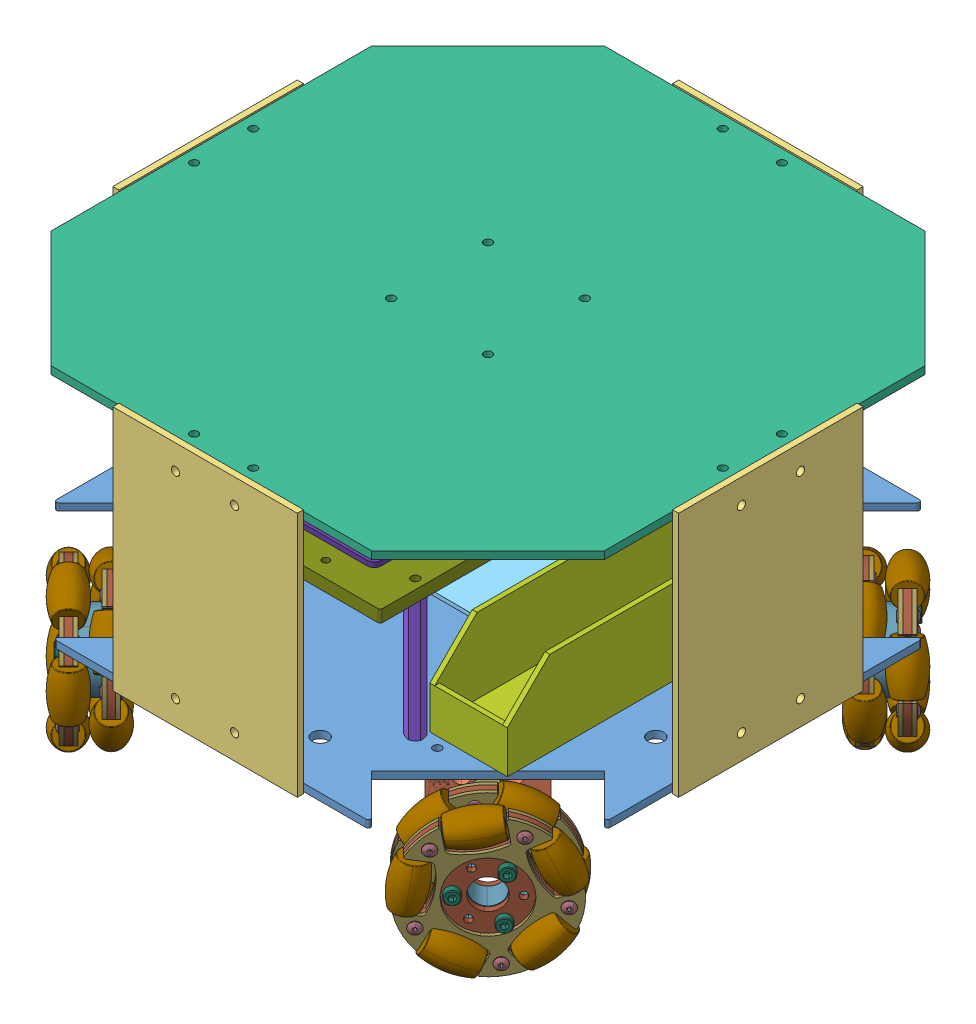
SolidWorks assembly ouijabot, configuration Default. Lengths in mm. (continued)
Components (placement in the parent): (continued)
- tx2-carrier-orbitty-1: tx2-carrier-orbitty [Default] at (43.5 74 -33.48) x (-1 0 0) z (0 -1 0) size (87.04 52.68 23.65) (continued)
  - ASG003_3D_MODEL.step-1: ASG003_3D_MODEL.step [Default] at origin size (87.04 52.68 23.65) (continued)
    - D8.step-1: D8.step [Default] at origin size (1.1 0.7 0.55) (continued)
      - 870944480.step-1: 870944480.step [Default] at (76.885 41.857 0) size (1.1 0.7 0.55) (continued)
        - Extruded-30.step-1: Extruded-30.step [Default] at origin size (1.1 0.7 0.55)
    - D7.step-1: D7.step [Default] at origin size (1 0.8 0.5)
      - 870940960.step-1: 870940960.step [Default] at (74.4974 43.1524 0) size (1 0.8 0.5)
        - Extruded-31.step-1: Extruded-31.step [Default] at origin size (1 0.8 0.5)
    - D6.step-1: D6.step [Default] at origin size (1 0.8 0.5)
      - 870940960.step-1: 870940960.step [Default] at (41.166 32.031 0) size (1 0.8 0.5)
        - Extruded-31.step-1: Extruded-31.step [Default] at origin size (1 0.8 0.5)
    - D5.step-1: D5.step [Default] at origin size (1 0.8 0.5)
      - 870940960.step-1: 870940960.step [Default] at (35.166 32.031 0) size (1 0.8 0.5)
        - Extruded-31.step-1: Extruded-31.step [Default] at origin size (1 0.8 0.5)
    - D4.step-1: D4.step [Default] at origin size (1 0.8 0.5)
      - 870940960.step-1: 870940960.step [Default] at (44.881 32.031 0) size (1 0.8 0.5)
        - Extruded-31.step-1: Extruded-31.step [Default] at origin size (1 0.8 0.5)
    - D2.step-1: D2.step [Default] at origin size (1.02 0.52 0.36)
      - 870944640.step-1: 870944640.step [Default] at (10.9212 1.0646 0) size (1.01 0.51 0.36)
        - Extruded-28.step-1: Extruded-28.step [Default] at origin size (1.01 0.51 0.36)
      - 870940480.step-1: 870940480.step [Default] at (10.4912 1.0646 0) size (0.16 0.52 0.35)
        - Extruded.step-1: Extruded.step [Default] at origin size (0.16 0.52 0.35)
      - 870940480.step-2: 870940480.step [Default] at (11.3512 1.0646 0) size (0.16 0.52 0.35)
        - Extruded.step-1: Extruded.step [Default] at origin size (0.16 0.52 0.35)
    - C57.step-1: C57.step [Default] at origin size (1.3 2.04 0.45)
      - 740904480.step-1: 740904480.step [Default] at (69.215 27.686 0) size (1.25 2 0.45)
        - Extruded-32.step-1: Extruded-32.step [Default] at origin size (1.25 2 0.45)
      - 740902240.step-1: 740902240.step [Default] at (69.215 26.7735 0) size (1.3 0.23 0.45)
        - Extruded-33.step-1: Extruded-33.step [Default] at origin size (1.3 0.23 0.45)
      - 740902240.step-2: 740902240.step [Default] at (69.215 28.586 0) size (1.3 0.23 0.45)
        - Extruded-33.step-1: Extruded-33.step [Default] at origin size (1.3 0.23 0.45)
    - C47.step-1: C47.step [Default] at origin size (1.3 2.04 0.45)
      - 740902240.step-1: 740902240.step [Default] at (72.8972 21.3736 0) size (1.3 0.23 0.45)
        - Extruded-33.step-1: Extruded-33.step [Default] at origin size (1.3 0.23 0.45)
      - 740902240.step-2: 740902240.step [Default] at (72.8972 23.1861 0) size (1.3 0.23 0.45)
        - Extruded-33.step-1: Extruded-33.step [Default] at origin size (1.3 0.23 0.45)
      - 740904480.step-1: 740904480.step [Default] at (72.8972 22.2736 0) size (1.25 2 0.45)
        - Extruded-32.step-1: Extruded-32.step [Default] at origin size (1.25 2 0.45)
    - C46.step-1: C46.step [Default] at origin size (1.3 2.04 0.45)
      - 740902240.step-1: 740902240.step [Default] at (76.9612 21.3736 0) size (1.3 0.23 0.45)
        - Extruded-33.step-1: Extruded-33.step [Default] at origin size (1.3 0.23 0.45)
      - 740902240.step-2: 740902240.step [Default] at (76.9612 23.1861 0) size (1.3 0.23 0.45)
        - Extruded-33.step-1: Extruded-33.step [Default] at origin size (1.3 0.23 0.45)
      - 740904480.step-1: 740904480.step [Default] at (76.9612 22.2736 0) size (1.25 2 0.45)
        - Extruded-32.step-1: Extruded-32.step [Default] at origin size (1.25 2 0.45)
    - C45.step-1: C45.step [Default] at origin size (1.3 2.04 0.45)
      - 740902240.step-1: 740902240.step [Default] at (74.9292 21.3736 0) size (1.3 0.23 0.45)
        - Extruded-33.step-1: Extruded-33.step [Default] at origin size (1.3 0.23 0.45)
      - 740902240.step-2: 740902240.step [Default] at (74.9292 23.1861 0) size (1.3 0.23 0.45)
        - Extruded-33.step-1: Extruded-33.step [Default] at origin size (1.3 0.23 0.45)
      - 740904480.step-1: 740904480.step [Default] at (74.9292 22.2736 0) size (1.25 2 0.45)
        - Extruded-32.step-1: Extruded-32.step [Default] at origin size (1.25 2 0.45)
    - C44.step-1: C44.step [Default] at origin size (1.02 0.52 0.36)
      - 870940480.step-1: 870940480.step [Default] at (29.084 26.6678 0) size (0.16 0.52 0.35)
        - Extruded.step-1: Extruded.step [Default] at origin size (0.16 0.52 0.35)
      - 870940480.step-2: 870940480.step [Default] at (29.944 26.6678 0) size (0.16 0.52 0.35)
        - Extruded.step-1: Extruded.step [Default] at origin size (0.16 0.52 0.35)
      - 870940640.step-1: 870940640.step [Default] at (29.514 26.6678 0) size (1.01 0.51 0.36)
        - Extruded-0.step-1: Extruded-0.step [Default] at origin size (1.01 0.51 0.36)
    - C43.step-1: C43.step [Default] at origin size (1.02 0.52 0.36)
      - 870940480.step-1: 870940480.step [Default] at (76.455 43 0) size (0.16 0.52 0.35)
        - Extruded.step-1: Extruded.step [Default] at origin size (0.16 0.52 0.35)
      - 870940480.step-2: 870940480.step [Default] at (77.315 43 0) size (0.16 0.52 0.35)
        - Extruded.step-1: Extruded.step [Default] at origin size (0.16 0.52 0.35)
      - 870940640.step-1: 870940640.step [Default] at (76.885 43 0) size (1.01 0.51 0.36)
        - Extruded-0.step-1: Extruded-0.step [Default] at origin size (1.01 0.51 0.36)
    - C42.step-1: C42.step [Default] at origin size (1.02 0.52 0.36)
      - 870940480.step-1: 870940480.step [Default] at (76.455 44.016 0) size (0.16 0.52 0.35)
        - Extruded.step-1: Extruded.step [Default] at origin size (0.16 0.52 0.35)
      - 870940480.step-2: 870940480.step [Default] at (77.315 44.016 0) size (0.16 0.52 0.35)
        - Extruded.step-1: Extruded.step [Default] at origin size (0.16 0.52 0.35)
      - 870940640.step-1: 870940640.step [Default] at (76.885 44.016 0) size (1.01 0.51 0.36)
        - Extruded-0.step-1: Extruded-0.step [Default] at origin size (1.01 0.51 0.36)
    - C41.step-1: C41.step [Default] at origin size (1.02 0.52 0.36)
      - 870940480.step-1: 870940480.step [Default] at (68.835 44.143 0) size (0.16 0.52 0.35)
        - Extruded.step-1: Extruded.step [Default] at origin size (0.16 0.52 0.35)
      - 870940480.step-2: 870940480.step [Default] at (69.695 44.143 0) size (0.16 0.52 0.35)
        - Extruded.step-1: Extruded.step [Default] at origin size (0.16 0.52 0.35)
      - 870940640.step-1: 870940640.step [Default] at (69.265 44.143 0) size (1.01 0.51 0.36)
        - Extruded-0.step-1: Extruded-0.step [Default] at origin size (1.01 0.51 0.36)
    - C40.step-1: C40.step [Default] at origin size (4.35 7.4 4.01)
      - 870941440.step-1: 870941440.step [Default] at (68.4522 37.8735 0) size (4.3 0.35 4.01)
        - Extruded-34.step-1: Extruded-34.step [Default] at origin size (4.3 0.35 4.01)
      - 870941600.step-1: 870941600.step [Default] at (68.4522 31.3736 0) size (2 0.2 2)
        - Extruded-35.step-1: Extruded-35.step [Default] at origin size (2 0.2 2)
      - 870941600.step-2: 870941600.step [Default] at (68.4522 38.5736 0) size (2 0.2 2)
        - Extruded-35.step-1: Extruded-35.step [Default] at origin size (2 0.2 2)
      - 870941760.step-1: 870941760.step [Default] at (68.4523 34.9735 0) size (4.35 7.3 4)
        - Extruded-36.step-1: Extruded-36.step [Default] at origin size (4.35 7.3 4)
    - C39.step-1: C39.step [Default] at origin size (1.02 0.52 0.36)
      - 870940480.step-1: 870940480.step [Default] at (39.673 40.1066 -1.9516) size (0.16 0.52 0.35)
        - Extruded.step-1: Extruded.step [Default] at origin size (0.16 0.52 0.35)
      - 870940480.step-2: 870940480.step [Default] at (38.813 40.1066 -1.9516) size (0.16 0.52 0.35)
        - Extruded.step-1: Extruded.step [Default] at origin size (0.16 0.52 0.35)
      - 870940640.step-1: 870940640.step [Default] at (39.243 40.1066 -1.9506) size (1.01 0.51 0.36)
        - Extruded-0.step-1: Extruded-0.step [Default] at origin size (1.01 0.51 0.36)
    - C38.step-1: C38.step [Default] at origin size (1.02 0.52 0.36)
      - 870940480.step-1: 870940480.step [Default] at (49.023 38.174 0) size (0.16 0.52 0.35)
        - Extruded.step-1: Extruded.step [Default] at origin size (0.16 0.52 0.35)
      - 870940480.step-2: 870940480.step [Default] at (49.883 38.174 0) size (0.16 0.52 0.35)
        - Extruded.step-1: Extruded.step [Default] at origin size (0.16 0.52 0.35)
      - 870940640.step-1: 870940640.step [Default] at (49.453 38.174 0) size (1.01 0.51 0.36)
        - Extruded-0.step-1: Extruded-0.step [Default] at origin size (1.01 0.51 0.36)
    - C37.step-1: C37.step [Default] at origin size (4.35 7.4 4.01)
      - 870941440.step-1: 870941440.step [Default] at (48.5132 35.3843 0) size (4.3 0.35 4.01)
        - Extruded-34.step-1: Extruded-34.step [Default] at origin size (4.3 0.35 4.01)
      - 870941600.step-1: 870941600.step [Default] at (48.5132 28.8844 0) size (2 0.2 2)
        - Extruded-35.step-1: Extruded-35.step [Default] at origin size (2 0.2 2)
      - 870941600.step-2: 870941600.step [Default] at (48.5132 36.0844 0) size (2 0.2 2)
        - Extruded-35.step-1: Extruded-35.step [Default] at origin size (2 0.2 2)
      - 870941760.step-1: 870941760.step [Default] at (48.5133 32.4843 0) size (4.35 7.3 4)
        - Extruded-36.step-1: Extruded-36.step [Default] at origin size (4.35 7.3 4)
    - C36.step-1: C36.step [Default] at origin size (0.52 1.02 0.36)
      - 870941120.step-1: 870941120.step [Default] at (41.666 26.961 0) size (0.52 0.16 0.35)
        - Extruded-1.step-1: Extruded-1.step [Default] at origin size (0.52 0.16 0.35)
      - 870941120.step-2: 870941120.step [Default] at (41.666 26.101 0) size (0.52 0.16 0.35)
        - Extruded-1.step-1: Extruded-1.step [Default] at origin size (0.52 0.16 0.35)
      - 870941280.step-1: 870941280.step [Default] at (41.666 26.531 0) size (0.51 1.01 0.36)
        - Extruded-2.step-1: Extruded-2.step [Default] at origin size (0.51 1.01 0.36)
    - C35.step-1: C35.step [Default] at origin size (0.52 1.02 0.36)
      - 870941120.step-1: 870941120.step [Default] at (40.666 26.961 0) size (0.52 0.16 0.35)
        - Extruded-1.step-1: Extruded-1.step [Default] at origin size (0.52 0.16 0.35)
      - 870941120.step-2: 870941120.step [Default] at (40.666 26.101 0) size (0.52 0.16 0.35)
        - Extruded-1.step-1: Extruded-1.step [Default] at origin size (0.52 0.16 0.35)
      - 870941280.step-1: 870941280.step [Default] at (40.666 26.531 0) size (0.51 1.01 0.36)
        - Extruded-2.step-1: Extruded-2.step [Default] at origin size (0.51 1.01 0.36)
    - C34.step-1: C34.step [Default] at origin size (1.02 0.52 0.36)
      - 870940480.step-1: 870940480.step [Default] at (83.0277 32.2771 -1.9516) size (0.16 0.52 0.35)
        - Extruded.step-1: Extruded.step [Default] at origin size (0.16 0.52 0.35)
      - 870940480.step-2: 870940480.step [Default] at (83.8877 32.2771 -1.9516) size (0.16 0.52 0.35)
        - Extruded.step-1: Extruded.step [Default] at origin size (0.16 0.52 0.35)
      - 870940640.step-1: 870940640.step [Default] at (83.4577 32.2771 -1.9506) size (1.01 0.51 0.36)
        - Extruded-0.step-1: Extruded-0.step [Default] at origin size (1.01 0.51 0.36)
    - C32.step-1: C32.step [Default] at origin size (0.52 1.02 0.36)
      - 870941120.step-1: 870941120.step [Default] at (22.148 19.554 -1.9516) size (0.52 0.16 0.35)
        - Extruded-1.step-1: Extruded-1.step [Default] at origin size (0.52 0.16 0.35)
      - 870941120.step-2: 870941120.step [Default] at (22.148 18.694 -1.9516) size (0.52 0.16 0.35)
        - Extruded-1.step-1: Extruded-1.step [Default] at origin size (0.52 0.16 0.35)
      - 870941280.step-1: 870941280.step [Default] at (22.148 19.124 -1.9506) size (0.51 1.01 0.36)
        - Extruded-2.step-1: Extruded-2.step [Default] at origin size (0.51 1.01 0.36)
    - C31.step-1: C31.step [Default] at origin size (0.52 1.02 0.36)
      - 870941120.step-1: 870941120.step [Default] at (11.607 19.554 -1.9516) size (0.52 0.16 0.35)
        - Extruded-1.step-1: Extruded-1.step [Default] at origin size (0.52 0.16 0.35)
      - 870941120.step-2: 870941120.step [Default] at (11.607 18.694 -1.9516) size (0.52 0.16 0.35)
        - Extruded-1.step-1: Extruded-1.step [Default] at origin size (0.52 0.16 0.35)
      - 870941280.step-1: 870941280.step [Default] at (11.607 19.124 -1.9506) size (0.51 1.01 0.36)
        - Extruded-2.step-1: Extruded-2.step [Default] at origin size (0.51 1.01 0.36)
    - C30.step-1: C30.step [Default] at origin size (0.52 1.02 0.36)
      - 870941120.step-1: 870941120.step [Default] at (14.147 19.623 -1.9516) size (0.52 0.16 0.35)
        - Extruded-1.step-1: Extruded-1.step [Default] at origin size (0.52 0.16 0.35)
      - 870941120.step-2: 870941120.step [Default] at (14.147 18.763 -1.9516) size (0.52 0.16 0.35)
        - Extruded-1.step-1: Extruded-1.step [Default] at origin size (0.52 0.16 0.35)
      - 870941280.step-1: 870941280.step [Default] at (14.147 19.193 -1.9506) size (0.51 1.01 0.36)
        - Extruded-2.step-1: Extruded-2.step [Default] at origin size (0.51 1.01 0.36)
    - C29.step-1: C29.step [Default] at origin size (1.02 0.52 0.36)
      - 870940480.step-1: 870940480.step [Default] at (25.528 26.617 -1.9516) size (0.16 0.52 0.35)
        - Extruded.step-1: Extruded.step [Default] at origin size (0.16 0.52 0.35)
      - 870940480.step-2: 870940480.step [Default] at (26.388 26.617 -1.9516) size (0.16 0.52 0.35)
        - Extruded.step-1: Extruded.step [Default] at origin size (0.16 0.52 0.35)
      - 870940640.step-1: 870940640.step [Default] at (25.958 26.617 -1.9506) size (1.01 0.51 0.36)
        - Extruded-0.step-1: Extruded-0.step [Default] at origin size (1.01 0.51 0.36)
    - C28.step-1: C28.step [Default] at origin size (1.02 0.52 0.36)
      - 870940480.step-1: 870940480.step [Default] at (25.782 24.077 -1.9516) size (0.16 0.52 0.35)
        - Extruded.step-1: Extruded.step [Default] at origin size (0.16 0.52 0.35)
      - 870940480.step-2: 870940480.step [Default] at (26.642 24.077 -1.9516) size (0.16 0.52 0.35)
        - Extruded.step-1: Extruded.step [Default] at origin size (0.16 0.52 0.35)
      - 870940640.step-1: 870940640.step [Default] at (26.212 24.077 -1.9506) size (1.01 0.51 0.36)
        - Extruded-0.step-1: Extruded-0.step [Default] at origin size (1.01 0.51 0.36)
    - C27.step-1: C27.step [Default] at origin size (1.02 0.52 0.36)
      - 870940480.step-1: 870940480.step [Default] at (10.0685 26.617 -1.9516) size (0.16 0.52 0.35)
        - Extruded.step-1: Extruded.step [Default] at origin size (0.16 0.52 0.35)
      - 870940480.step-2: 870940480.step [Default] at (9.2085 26.617 -1.9516) size (0.16 0.52 0.35)
        - Extruded.step-1: Extruded.step [Default] at origin size (0.16 0.52 0.35)
      - 870940640.step-1: 870940640.step [Default] at (9.6385 26.617 -1.9506) size (1.01 0.51 0.36)
        - Extruded-0.step-1: Extruded-0.step [Default] at origin size (1.01 0.51 0.36)
    - C26.step-1: C26.step [Default] at origin size (1.02 0.52 0.36)
      - 870940480.step-1: 870940480.step [Default] at (9.878 24.077 -1.9516) size (0.16 0.52 0.35)
        - Extruded.step-1: Extruded.step [Default] at origin size (0.16 0.52 0.35)
      - 870940480.step-2: 870940480.step [Default] at (9.018 24.077 -1.9516) size (0.16 0.52 0.35)
        - Extruded.step-1: Extruded.step [Default] at origin size (0.16 0.52 0.35)
      - 870940640.step-1: 870940640.step [Default] at (9.448 24.077 -1.9506) size (1.01 0.51 0.36)
        - Extruded-0.step-1: Extruded-0.step [Default] at origin size (1.01 0.51 0.36)
    - C25.step-1: C25.step [Default] at origin size (1.02 0.52 0.36)
      - 870940480.step-1: 870940480.step [Default] at (7.923 33.147 -1.9516) size (0.16 0.52 0.35)
        - Extruded.step-1: Extruded.step [Default] at origin size (0.16 0.52 0.35)
      - 870940480.step-2: 870940480.step [Default] at (7.063 33.147 -1.9516) size (0.16 0.52 0.35)
        - Extruded.step-1: Extruded.step [Default] at origin size (0.16 0.52 0.35)
      - 870940640.step-1: 870940640.step [Default] at (7.493 33.147 -1.9506) size (1.01 0.51 0.36)
        - Extruded-0.step-1: Extruded-0.step [Default] at origin size (1.01 0.51 0.36)
    - C24.step-1: C24.step [Default] at origin size (1.02 0.52 0.36)
      - 870940480.step-1: 870940480.step [Default] at (9.603 33.147 -1.9516) size (0.16 0.52 0.35)
        - Extruded.step-1: Extruded.step [Default] at origin size (0.16 0.52 0.35)
      - 870940480.step-2: 870940480.step [Default] at (10.463 33.147 -1.9516) size (0.16 0.52 0.35)
        - Extruded.step-1: Extruded.step [Default] at origin size (0.16 0.52 0.35)
      - 870940640.step-1: 870940640.step [Default] at (10.033 33.147 -1.9506) size (1.01 0.51 0.36)
        - Extruded-0.step-1: Extruded-0.step [Default] at origin size (1.01 0.51 0.36)
    - C23.step-1: C23.step [Default] at origin size (1.3 2.04 0.45)
      - 740904480.step-1: 740904480.step [Default] at (78.486 26.162 -2.0506) size (1.25 2 0.45)
        - Extruded-32.step-1: Extruded-32.step [Default] at origin size (1.25 2 0.45)
      - 740902240.step-1: 740902240.step [Default] at (78.486 27.0745 -2.0516) size (1.3 0.23 0.45)
        - Extruded-33.step-1: Extruded-33.step [Default] at origin size (1.3 0.23 0.45)
      - 740902240.step-2: 740902240.step [Default] at (78.486 25.262 -2.0516) size (1.3 0.23 0.45)
        - Extruded-33.step-1: Extruded-33.step [Default] at origin size (1.3 0.23 0.45)
    - C22.step-1: C22.step [Default] at origin size (0.52 1.02 0.36)
      - 870941120.step-1: 870941120.step [Default] at (7.493 41.099 -1.9516) size (0.52 0.16 0.35)
        - Extruded-1.step-1: Extruded-1.step [Default] at origin size (0.52 0.16 0.35)
      - 870941120.step-2: 870941120.step [Default] at (7.493 41.959 -1.9516) size (0.52 0.16 0.35)
        - Extruded-1.step-1: Extruded-1.step [Default] at origin size (0.52 0.16 0.35)
      - 870941280.step-1: 870941280.step [Default] at (7.493 41.529 -1.9506) size (0.51 1.01 0.36)
        - Extruded-2.step-1: Extruded-2.step [Default] at origin size (0.51 1.01 0.36)
    - C21.step-1: C21.step [Default] at origin size (0.52 1.02 0.36)
      - 870941120.step-1: 870941120.step [Default] at (8.636 41.099 -1.9516) size (0.52 0.16 0.35)
        - Extruded-1.step-1: Extruded-1.step [Default] at origin size (0.52 0.16 0.35)
      - 870941120.step-2: 870941120.step [Default] at (8.636 41.959 -1.9516) size (0.52 0.16 0.35)
        - Extruded-1.step-1: Extruded-1.step [Default] at origin size (0.52 0.16 0.35)
      - 870941280.step-1: 870941280.step [Default] at (8.636 41.529 -1.9506) size (0.51 1.01 0.36)
        - Extruded-2.step-1: Extruded-2.step [Default] at origin size (0.51 1.01 0.36)
    - C19.step-1: C19.step [Default] at origin size (1.6 0.9 0.46)
      - 870942080.step-1: 870942080.step [Default] at (62.892 37.465 0) size (0.3 0.9 0.46)
        - Extruded-13.step-1: Extruded-13.step [Default] at origin size (0.3 0.9 0.46)
      - 870942080.step-2: 870942080.step [Default] at (61.592 37.465 0) size (0.3 0.9 0.46)
        - Extruded-13.step-1: Extruded-13.step [Default] at origin size (0.3 0.9 0.46)
      - 870942240.step-1: 870942240.step [Default] at (62.242 37.465 0) size (1 0.9 0.45)
        - Extruded-12.step-1: Extruded-12.step [Default] at origin size (1 0.9 0.45)
    - C18.step-1: C18.step [Default] at origin size (1.02 0.52 0.36)
      - 870940480.step-1: 870940480.step [Default] at (53.722 33.3988 -1.9516) size (0.16 0.52 0.35)
        - Extruded.step-1: Extruded.step [Default] at origin size (0.16 0.52 0.35)
      - 870940480.step-2: 870940480.step [Default] at (54.582 33.3988 -1.9516) size (0.16 0.52 0.35)
        - Extruded.step-1: Extruded.step [Default] at origin size (0.16 0.52 0.35)
      - 870940640.step-1: 870940640.step [Default] at (54.152 33.3988 -1.9506) size (1.01 0.51 0.36)
        - Extruded-0.step-1: Extruded-0.step [Default] at origin size (1.01 0.51 0.36)
    - C17.step-1: C17.step [Default] at origin size (1.02 0.52 0.36)
      - 870940480.step-1: 870940480.step [Default] at (57.7824 32.2304 -1.9516) size (0.16 0.52 0.35)
        - Extruded.step-1: Extruded.step [Default] at origin size (0.16 0.52 0.35)
      - 870940480.step-2: 870940480.step [Default] at (56.9224 32.2304 -1.9516) size (0.16 0.52 0.35)
        - Extruded.step-1: Extruded.step [Default] at origin size (0.16 0.52 0.35)
      - 870940640.step-1: 870940640.step [Default] at (57.3524 32.2304 -1.9506) size (1.01 0.51 0.36)
        - Extruded-0.step-1: Extruded-0.step [Default] at origin size (1.01 0.51 0.36)
    - C16.step-1: C16.step [Default] at origin size (1.02 0.52 0.36)
      - 870940480.step-1: 870940480.step [Default] at (54.582 34.6434 -1.9516) size (0.16 0.52 0.35)
        - Extruded.step-1: Extruded.step [Default] at origin size (0.16 0.52 0.35)
      - 870940480.step-2: 870940480.step [Default] at (53.722 34.6434 -1.9516) size (0.16 0.52 0.35)
        - Extruded.step-1: Extruded.step [Default] at origin size (0.16 0.52 0.35)
      - 870940640.step-1: 870940640.step [Default] at (54.152 34.6434 -1.9506) size (1.01 0.51 0.36)
        - Extruded-0.step-1: Extruded-0.step [Default] at origin size (1.01 0.51 0.36)
    - C15.step-1: C15.step [Default] at origin size (0.52 1.02 0.36)
      - 870941120.step-1: 870941120.step [Default] at (51.6628 25.4722 0) size (0.52 0.16 0.35)
        - Extruded-1.step-1: Extruded-1.step [Default] at origin size (0.52 0.16 0.35)
      - 870941120.step-2: 870941120.step [Default] at (51.6628 24.6122 0) size (0.52 0.16 0.35)
        - Extruded-1.step-1: Extruded-1.step [Default] at origin size (0.52 0.16 0.35)
      - 870941280.step-1: 870941280.step [Default] at (51.6628 25.0422 0) size (0.51 1.01 0.36)
        - Extruded-2.step-1: Extruded-2.step [Default] at origin size (0.51 1.01 0.36)
    - C14.step-1: C14.step [Default] at origin size (0.52 1.02 0.36)
      - 870941120.step-1: 870941120.step [Default] at (50.6468 25.4722 0) size (0.52 0.16 0.35)
        - Extruded-1.step-1: Extruded-1.step [Default] at origin size (0.52 0.16 0.35)
      - 870941120.step-2: 870941120.step [Default] at (50.6468 24.6122 0) size (0.52 0.16 0.35)
        - Extruded-1.step-1: Extruded-1.step [Default] at origin size (0.52 0.16 0.35)
      - 870941280.step-1: 870941280.step [Default] at (50.6468 25.0422 0) size (0.51 1.01 0.36)
        - Extruded-2.step-1: Extruded-2.step [Default] at origin size (0.51 1.01 0.36)
    - C13.step-1: C13.step [Default] at origin size (0.52 1.02 0.36)
      - 870941120.step-1: 870941120.step [Default] at (54.4568 26.4882 0) size (0.52 0.16 0.35)
        - Extruded-1.step-1: Extruded-1.step [Default] at origin size (0.52 0.16 0.35)
      - 870941120.step-2: 870941120.step [Default] at (54.4568 25.6282 0) size (0.52 0.16 0.35)
        - Extruded-1.step-1: Extruded-1.step [Default] at origin size (0.52 0.16 0.35)
      - 870941280.step-1: 870941280.step [Default] at (54.4568 26.0582 0) size (0.51 1.01 0.36)
        - Extruded-2.step-1: Extruded-2.step [Default] at origin size (0.51 1.01 0.36)
    - C12.step-1: C12.step [Default] at origin size (0.52 1.02 0.36)
      - 870941120.step-1: 870941120.step [Default] at (53.4408 26.4882 0) size (0.52 0.16 0.35)
        - Extruded-1.step-1: Extruded-1.step [Default] at origin size (0.52 0.16 0.35)
      - 870941120.step-2: 870941120.step [Default] at (53.4408 25.6282 0) size (0.52 0.16 0.35)
        - Extruded-1.step-1: Extruded-1.step [Default] at origin size (0.52 0.16 0.35)
      - 870941280.step-1: 870941280.step [Default] at (53.4408 26.0582 0) size (0.51 1.01 0.36)
        - Extruded-2.step-1: Extruded-2.step [Default] at origin size (0.51 1.01 0.36)
    - C11.step-1: C11.step [Default] at origin size (0.52 1.02 0.36)
      - 870941120.step-1: 870941120.step [Default] at (57.2508 25.4722 0) size (0.52 0.16 0.35)
        - Extruded-1.step-1: Extruded-1.step [Default] at origin size (0.52 0.16 0.35)
      - 870941120.step-2: 870941120.step [Default] at (57.2508 24.6122 0) size (0.52 0.16 0.35)
        - Extruded-1.step-1: Extruded-1.step [Default] at origin size (0.52 0.16 0.35)
      - 870941280.step-1: 870941280.step [Default] at (57.2508 25.0422 0) size (0.51 1.01 0.36)
        - Extruded-2.step-1: Extruded-2.step [Default] at origin size (0.51 1.01 0.36)
    - C10.step-1: C10.step [Default] at origin size (0.52 1.02 0.36)
      - 870941120.step-1: 870941120.step [Default] at (56.2348 25.4722 0) size (0.52 0.16 0.35)
        - Extruded-1.step-1: Extruded-1.step [Default] at origin size (0.52 0.16 0.35)
      - 870941120.step-2: 870941120.step [Default] at (56.2348 24.6122 0) size (0.52 0.16 0.35)
        - Extruded-1.step-1: Extruded-1.step [Default] at origin size (0.52 0.16 0.35)
      - 870941280.step-1: 870941280.step [Default] at (56.2348 25.0422 0) size (0.51 1.01 0.36)
        - Extruded-2.step-1: Extruded-2.step [Default] at origin size (0.51 1.01 0.36)
    - C9.step-1: C9.step [Default] at origin size (0.52 1.02 0.36)
      - 870941120.step-1: 870941120.step [Default] at (60.0448 26.4882 0) size (0.52 0.16 0.35)
        - Extruded-1.step-1: Extruded-1.step [Default] at origin size (0.52 0.16 0.35)
      - 870941120.step-2: 870941120.step [Default] at (60.0448 25.6282 0) size (0.52 0.16 0.35)
        - Extruded-1.step-1: Extruded-1.step [Default] at origin size (0.52 0.16 0.35)
      - 870941280.step-1: 870941280.step [Default] at (60.0448 26.0582 0) size (0.51 1.01 0.36)
        - Extruded-2.step-1: Extruded-2.step [Default] at origin size (0.51 1.01 0.36)
    - C8.step-1: C8.step [Default] at origin size (0.52 1.02 0.36)
      - 870941120.step-1: 870941120.step [Default] at (59.0288 26.4882 0) size (0.52 0.16 0.35)
        - Extruded-1.step-1: Extruded-1.step [Default] at origin size (0.52 0.16 0.35)
      - 870941120.step-2: 870941120.step [Default] at (59.0288 25.6282 0) size (0.52 0.16 0.35)
        - Extruded-1.step-1: Extruded-1.step [Default] at origin size (0.52 0.16 0.35)
      - 870941280.step-1: 870941280.step [Default] at (59.0288 26.0582 0) size (0.51 1.01 0.36)
        - Extruded-2.step-1: Extruded-2.step [Default] at origin size (0.51 1.01 0.36)
    - C6.step-1: C6.step [Default] at origin size (1.6 0.9 0.46)
      - 870942080.step-1: 870942080.step [Default] at (72.7044 4.138 0) size (0.3 0.9 0.46)
        - Extruded-13.step-1: Extruded-13.step [Default] at origin size (0.3 0.9 0.46)
      - 870942080.step-2: 870942080.step [Default] at (74.0044 4.138 0) size (0.3 0.9 0.46)
        - Extruded-13.step-1: Extruded-13.step [Default] at origin size (0.3 0.9 0.46)
      - 870942240.step-1: 870942240.step [Default] at (73.3544 4.138 0) size (1 0.9 0.45)
        - Extruded-12.step-1: Extruded-12.step [Default] at origin size (1 0.9 0.45)
    - C5.step-1: C5.step [Default] at origin size (1.6 0.9 0.46)
      - 870942080.step-1: 870942080.step [Default] at (72.7044 5.4842 0) size (0.3 0.9 0.46)
        - Extruded-13.step-1: Extruded-13.step [Default] at origin size (0.3 0.9 0.46)
      - 870942080.step-2: 870942080.step [Default] at (74.0044 5.4842 0) size (0.3 0.9 0.46)
        - Extruded-13.step-1: Extruded-13.step [Default] at origin size (0.3 0.9 0.46)
      - 870942240.step-1: 870942240.step [Default] at (73.3544 5.4842 0) size (1 0.9 0.45)
        - Extruded-12.step-1: Extruded-12.step [Default] at origin size (1 0.9 0.45)
    - C4.step-1: C4.step [Default] at origin size (2.04 1.3 0.45)
      - 870943200.step-1: 870943200.step [Default] at (77.139 5.5604 0) size (2 1.25 0.45)
        - Extruded-37.step-1: Extruded-37.step [Default] at origin size (2 1.25 0.45)
      - 870943360.step-1: 870943360.step [Default] at (78.0515 5.5604 0) size (0.23 1.3 0.45)
        - Extruded-38.step-1: Extruded-38.step [Default] at origin size (0.23 1.3 0.45)
      - 870943360.step-2: 870943360.step [Default] at (76.239 5.5604 0) size (0.23 1.3 0.45)
        - Extruded-38.step-1: Extruded-38.step [Default] at origin size (0.23 1.3 0.45)
    - C3.step-1: C3.step [Default] at origin size (1.3 2.04 0.45)
      - 740904480.step-1: 740904480.step [Default] at (76.3008 2.8426 0) size (1.25 2 0.45)
        - Extruded-32.step-1: Extruded-32.step [Default] at origin size (1.25 2 0.45)
      - 740902240.step-1: 740902240.step [Default] at (76.3008 1.9301 0) size (1.3 0.23 0.45)
        - Extruded-33.step-1: Extruded-33.step [Default] at origin size (1.3 0.23 0.45)
      - 740902240.step-2: 740902240.step [Default] at (76.3008 3.7426 0) size (1.3 0.23 0.45)
        - Extruded-33.step-1: Extruded-33.step [Default] at origin size (1.3 0.23 0.45)
    - C2.step-1: C2.step [Default] at origin size (2.04 1.3 0.45)
      - 870943200.step-1: 870943200.step [Default] at (73.3798 2.4108 0) size (2 1.25 0.45)
        - Extruded-37.step-1: Extruded-37.step [Default] at origin size (2 1.25 0.45)
      - 870943360.step-1: 870943360.step [Default] at (72.4673 2.4108 0) size (0.23 1.3 0.45)
        - Extruded-38.step-1: Extruded-38.step [Default] at origin size (0.23 1.3 0.45)
      - 870943360.step-2: 870943360.step [Default] at (74.2798 2.4108 0) size (0.23 1.3 0.45)
        - Extruded-38.step-1: Extruded-38.step [Default] at origin size (0.23 1.3 0.45)
    - C1.step-1: C1.step [Default] at origin size (2.04 1.3 0.45)
      - 870943200.step-1: 870943200.step [Default] at (73.3544 7.1606 0) size (2 1.25 0.45)
        - Extruded-37.step-1: Extruded-37.step [Default] at origin size (2 1.25 0.45)
      - 870943360.step-1: 870943360.step [Default] at (72.4419 7.1606 0) size (0.23 1.3 0.45)
        - Extruded-38.step-1: Extruded-38.step [Default] at origin size (0.23 1.3 0.45)
      - 870943360.step-2: 870943360.step [Default] at (74.2544 7.1606 0) size (0.23 1.3 0.45)
        - Extruded-38.step-1: Extruded-38.step [Default] at origin size (0.23 1.3 0.45)
    - P1.step-1: P1.step [Default] at origin size (69.37 12.14 8.38)
      - SEAM-50-03.5-S-08-2-A-K-TR.step-1: SEAM-50-03.5-S-08-2-A-K-TR.step [Default] at (43.4999 7.4255 -4.9661) x (1 0 0) z (0 1 0) size (69.37 8.38 12.14)
        - _SEAM-50-03.5-L-08-1-A-K-TR_body.step-1: _SEAM-50-03.5-L-08-1-A-K-TR_body.step [Default] at origin size (69.37 8.38 12.14)
        - _SEAM-50-03.5-L-08-1-A-K-TR_conn.step-1: _SEAM-50-03.5-L-08-1-A-K-TR_conn.step [Default] at origin size (67.97 5.75 11.63)
        - _SEAM_K_Pad_08.step-1: _SEAM_K_Pad_08.step [Default] at (0 2.7432 0) size (8.26 0.13 8.26)
        - _SEAM_Triangle.step-1: _SEAM_Triangle.step [Default] at (32.2834 1.3462 -4.2164) x (-1 0 0) z (0 0 -1) size (1.02 1.27 0.13)
    - C51.step-1: C51.step [Default] at origin size (2.04 1.3 0.45)
      - 870943360.step-1: 870943360.step [Default] at (63.4848 22.2482 0) size (0.23 1.3 0.45)
        - Extruded-38.step-1: Extruded-38.step [Default] at origin size (0.23 1.3 0.45)
      - 870943360.step-2: 870943360.step [Default] at (61.6723 22.2482 0) size (0.23 1.3 0.45)
        - Extruded-38.step-1: Extruded-38.step [Default] at origin size (0.23 1.3 0.45)
      - 870943200.step-1: 870943200.step [Default] at (62.5848 22.2482 0) size (2 1.25 0.45)
        - Extruded-37.step-1: Extruded-37.step [Default] at origin size (2 1.25 0.45)
    - C52.step-1: C52.step [Default] at origin size (1.3 2.04 0.45)
      - 740902240.step-1: 740902240.step [Default] at (69.5952 17.9666 0) size (1.3 0.23 0.45)
        - Extruded-33.step-1: Extruded-33.step [Default] at origin size (1.3 0.23 0.45)
      - 740902240.step-2: 740902240.step [Default] at (69.5952 16.1541 0) size (1.3 0.23 0.45)
        - Extruded-33.step-1: Extruded-33.step [Default] at origin size (1.3 0.23 0.45)
      - 740904480.step-1: 740904480.step [Default] at (69.5952 17.0666 0) size (1.25 2 0.45)
        - Extruded-32.step-1: Extruded-32.step [Default] at origin size (1.25 2 0.45)
    - C53.step-1: C53.step [Default] at origin size (1.3 2.04 0.45)
      - 740902240.step-1: 740902240.step [Default] at (59.1812 17.9666 0) size (1.3 0.23 0.45)
        - Extruded-33.step-1: Extruded-33.step [Default] at origin size (1.3 0.23 0.45)
      - 740902240.step-2: 740902240.step [Default] at (59.1812 16.1541 0) size (1.3 0.23 0.45)
        - Extruded-33.step-1: Extruded-33.step [Default] at origin size (1.3 0.23 0.45)
      - 740904480.step-1: 740904480.step [Default] at (59.1812 17.0666 0) size (1.25 2 0.45)
        - Extruded-32.step-1: Extruded-32.step [Default] at origin size (1.25 2 0.45)
    - C54.step-1: C54.step [Default] at origin size (2.04 1.3 0.45)
      - 870943360.step-1: 870943360.step [Default] at (65.3678 22.2482 0) size (0.23 1.3 0.45)
        - Extruded-38.step-1: Extruded-38.step [Default] at origin size (0.23 1.3 0.45)
      - 870943360.step-2: 870943360.step [Default] at (67.1803 22.2482 0) size (0.23 1.3 0.45)
        - Extruded-38.step-1: Extruded-38.step [Default] at origin size (0.23 1.3 0.45)
      - 870943200.step-1: 870943200.step [Default] at (66.2678 22.2482 0) size (2 1.25 0.45)
        - Extruded-37.step-1: Extruded-37.step [Default] at origin size (2 1.25 0.45)
    - C55.step-1: C55.step [Default] at origin size (1.02 0.52 0.36)
      - 870940640.step-1: 870940640.step [Default] at (61.3982 17.1936 -1.9506) size (1.01 0.51 0.36)
        - Extruded-0.step-1: Extruded-0.step [Default] at origin size (1.01 0.51 0.36)
      - 870940480.step-1: 870940480.step [Default] at (60.9682 17.1936 -1.9516) size (0.16 0.52 0.35)
        - Extruded.step-1: Extruded.step [Default] at origin size (0.16 0.52 0.35)
      - 870940480.step-2: 870940480.step [Default] at (61.8282 17.1936 -1.9516) size (0.16 0.52 0.35)
        - Extruded.step-1: Extruded.step [Default] at origin size (0.16 0.52 0.35)
    - C56.step-1: C56.step [Default] at origin size (1.02 0.52 0.36)
      - 870940640.step-1: 870940640.step [Default] at (67.6648 17.219 -1.9506) size (1.01 0.51 0.36)
        - Extruded-0.step-1: Extruded-0.step [Default] at origin size (1.01 0.51 0.36)
      - 870940480.step-1: 870940480.step [Default] at (68.0948 17.219 -1.9516) size (0.16 0.52 0.35)
        - Extruded.step-1: Extruded.step [Default] at origin size (0.16 0.52 0.35)
      - 870940480.step-2: 870940480.step [Default] at (67.2348 17.219 -1.9516) size (0.16 0.52 0.35)
        - Extruded.step-1: Extruded.step [Default] at origin size (0.16 0.52 0.35)
    - R41.step-1: R41.step [Default] at origin size (1.02 0.52 0.36)
      - 870940640.step-1: 870940640.step [Default] at (67.6648 15.9744 -1.9506) size (1.01 0.51 0.36)
        - Extruded-0.step-1: Extruded-0.step [Default] at origin size (1.01 0.51 0.36)
      - 870940480.step-1: 870940480.step [Default] at (67.2348 15.9744 -1.9516) size (0.16 0.52 0.35)
        - Extruded.step-1: Extruded.step [Default] at origin size (0.16 0.52 0.35)
      - 870940480.step-2: 870940480.step [Default] at (68.0948 15.9744 -1.9516) size (0.16 0.52 0.35)
        - Extruded.step-1: Extruded.step [Default] at origin size (0.16 0.52 0.35)
    - R42.step-1: R42.step [Default] at origin size (1.02 0.52 0.36)
      - 870940640.step-1: 870940640.step [Default] at (61.3982 15.9236 -1.9506) size (1.01 0.51 0.36)
        - Extruded-0.step-1: Extruded-0.step [Default] at origin size (1.01 0.51 0.36)
      - 870940480.step-1: 870940480.step [Default] at (61.8282 15.9236 -1.9516) size (0.16 0.52 0.35)
        - Extruded.step-1: Extruded.step [Default] at origin size (0.16 0.52 0.35)
      - 870940480.step-2: 870940480.step [Default] at (60.9682 15.9236 -1.9516) size (0.16 0.52 0.35)
        - Extruded.step-1: Extruded.step [Default] at origin size (0.16 0.52 0.35)
    - R43.step-1: R43.step [Default] at origin size (0.52 1.02 0.36)
      - 870941280.step-1: 870941280.step [Default] at (64.3882 15.4736 -1.9506) size (0.51 1.01 0.36)
        - Extruded-2.step-1: Extruded-2.step [Default] at origin size (0.51 1.01 0.36)
      - 870941120.step-1: 870941120.step [Default] at (64.3882 15.9036 -1.9516) size (0.52 0.16 0.35)
        - Extruded-1.step-1: Extruded-1.step [Default] at origin size (0.52 0.16 0.35)
      - 870941120.step-2: 870941120.step [Default] at (64.3882 15.0436 -1.9516) size (0.52 0.16 0.35)
        - Extruded-1.step-1: Extruded-1.step [Default] at origin size (0.52 0.16 0.35)
    - U6.step-1: U6.step [Default] at origin size (6.25 6.25 1.55)
      - 870945760.step-1: 870945760.step [Default] at (64.3882 17.1936 0.37) size (6.25 6.25 1.55)
        - Extruded-39.step-1: Extruded-39.step [Default] at origin size (6.25 6.25 1.55)
    - Q7.step-1: Q7.step [Default] at origin size (2.9 2.42 1)
      - SW3dPS-SOT-23.step-1: SW3dPS-SOT-23.step [Default] at (67.8839 8.593 0.498) x (0 -1 0) z (-1 0 0) size (2.42 1 2.9)
    - P9.step-1: P9.step [Default] at origin size (7.3 7 12)
      - c-1546551-2-a-3d_RGB52224.step-1: c-1546551-2-a-3d_RGB52224.step [Default] at (86.8889 13.8152 2.4127) x (0 1 0) z (1 0 0) size (7 12 7.3)
    - Board.step-1: Board.step [Default] at (0 0 -1.6006) size (87 50 1.6)
